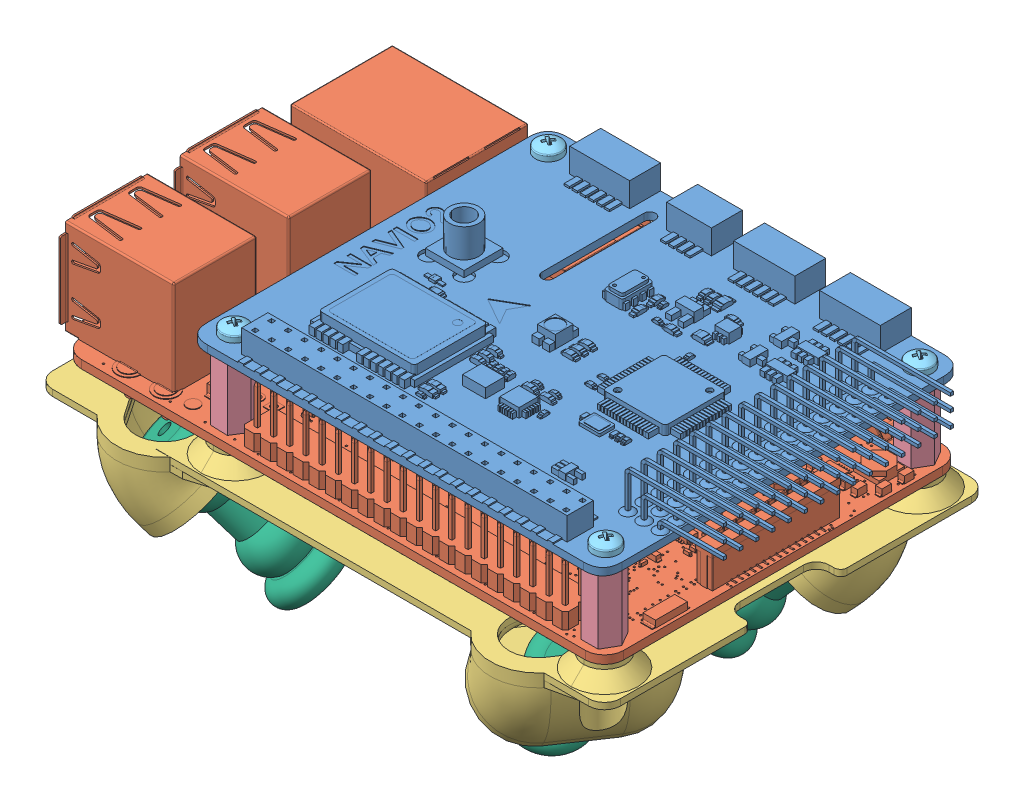
SolidWorks assembly FlightControllerAssembly, configuration Default. Lengths in mm.
Overall size (95.83 50.79 65.38).
19 component instances, 6 part files, 45 mates.
Components (placement in the parent):
- Navio2-1: Navio2 [Predeterminado] at origin size (73.82 8.2 56.43)
- raspberryPi3B-1: raspberryPi3B [Detailed] at (-9.9807 -13.4 -0.0405) x (-1 0 0) z (0 1 0) size (87.05 58.5 19.05)
- VibroNavio2top_rev_A-1: VibroNavio2top_rev_A [Default] at (-9.9807 -17.4 -0.0405) size (89 17.02 65.38)
- Spacer-1: Spacer [Default] at (29.0193 -12.1 24.4595) size (5.4 10.95 4.68)
- Spacer-2: Spacer [Default] at (-28.9807 -12.1 24.4595) x (0.999395 0 0.034774) z (-0.034774 0 0.999395) size (5.4 10.95 4.68)
- Spacer-3: Spacer [Default] at (-28.9807 -12.1 -24.5405) size (5.4 10.95 4.68)
- Spacer-4: Spacer [Default] at (29.0193 -12.1 -24.5405) size (5.4 10.95 4.68)
- pan cross head_am-1: pan cross head_am [B18.6.7M - M2 x 0.4 x 6 Type I Cross Recessed PHMS --6N] at (-28.9807 -17 24.4595) x (0 1 0) z (0 0 1) size (7.58 4 4)
- pan cross head_am-2: pan cross head_am [B18.6.7M - M2 x 0.4 x 6 Type I Cross Recessed PHMS --6N] at (-28.9807 -17 -24.5405) x (0 1 0) z (0 0 1) size (7.58 4 4)
- pan cross head_am-3: pan cross head_am [B18.6.7M - M2 x 0.4 x 6 Type I Cross Recessed PHMS --6N] at (-28.9807 1.6 -24.7405) x (0 -1 0) z (-0.546944 0 0.837169) size (7.58 4 4)
- pan cross head_am-4: pan cross head_am [B18.6.7M - M2 x 0.4 x 6 Type I Cross Recessed PHMS --6N] at (29.0193 -17 -24.5405) x (0 1 0) z (0 0 1) size (7.58 4 4)
- pan cross head_am-5: pan cross head_am [B18.6.7M - M2 x 0.4 x 6 Type I Cross Recessed PHMS --6N] at (29.2193 1.6 -24.7405) x (0 -1 0) z (-0.546944 0 0.837169) size (7.58 4 4)
- pan cross head_am-6: pan cross head_am [B18.6.7M - M2 x 0.4 x 6 Type I Cross Recessed PHMS --6N] at (29.0193 -17 24.4595) x (0 1 0) z (0 0 1) size (7.58 4 4)
- pan cross head_am-7: pan cross head_am [B18.6.7M - M2 x 0.4 x 6 Type I Cross Recessed PHMS --6N] at (29.2193 1.6 24.4595) x (0 -1 0) z (-0.546944 0 0.837169) size (7.58 4 4)
- pan cross head_am-8: pan cross head_am [B18.6.7M - M2 x 0.4 x 6 Type I Cross Recessed PHMS --6N] at (-28.9807 1.6 24.4595) x (0 -1 0) z (-0.546944 0 0.837169) size (7.58 4 4)
- DampeningBall-1: DampeningBall [Default] at (-27.8836 -38.7643 -12.0305) x (0.809631 0.541117 -0.227355) z (-0.054659 0.455184 0.888718) size (12 25 12)
- DampeningBall-2: DampeningBall [Default] at (-27.8836 -38.7643 11.9496) x (0.585019 0.027134 0.810565) z (-0.562354 -0.706586 0.429528) size (12 25 12)
- DampeningBall-3: DampeningBall [Default] at (7.693 -38.5525 11.8752) x (0.798628 -0.586314 -0.135756) z (-0.135756 -0.395268 0.908479) size (12 25 12)
- DampeningBall-4: DampeningBall [Default] at (7.693 -38.5525 -11.9561) x (0.662805 -0.699271 -0.267787) z (0.465753 0.104978 0.878666) size (12 25 12)
Mates (geometry in assembly coordinates):
- Coincident9: coincident aligned: plane of Navio2-1 through (0 0 0) normal (0 0 1)
- Coincident10: coincident aligned: plane of Navio2-1 through (0 0 0) normal (0 1 0)
- Coincident11: coincident aligned: plane of Navio2-1 through (0 0 0) normal (1 0 0)
- Parallel1: parallel aligned: plane of raspberryPi3B-1 through (-9.9807 -13.4 -0.0405) normal (0 1 0)
- Concentric5: concentric aligned: cylinder of Navio2-1 through (-28.9807 -1.166 24.4595) axis (0 1 0) radius 1.3; cylinder of raspberryPi3B-1 through (-28.9807 -13.4 24.4595) axis (0 1 0) radius 1.375
- Parallel3: parallel aligned: plane of Navio2-1 through (-32.5 -1.15 -28.2) normal (0 0 -1); plane of raspberryPi3B-1 through (32.5193 -12.1 -28.0405) normal (0 0 -1)
- Concentric7: concentric anti-aligned: cylinder of raspberryPi3B-1 through (29.0193 -13.4 24.4595) axis (0 1 0) radius 1.375; cylinder of VibroNavio2top_rev_A-1 through (29.0193 -16.4 24.4595) axis (0 -1 0) radius 1.5
- Concentric8: concentric anti-aligned: cylinder of raspberryPi3B-1 through (-28.9807 -13.4 -24.5405) axis (0 1 0) radius 1.375; cylinder of VibroNavio2top_rev_A-1 through (-28.9807 -16.4 -24.5405) axis (0 -1 0) radius 1.5
- Coincident15: coincident anti-aligned: plane of raspberryPi3B-1 through (-9.9807 -13.4 -0.0405) normal (0 -1 0); plane of VibroNavio2top_rev_A-1 through (29.0193 -13.4 -24.5405) normal (0 1 0)
- Concentric9: concentric aligned: cylinder of raspberryPi3B-1 through (-28.9807 -13.4 24.4595) axis (0 1 0) radius 1.375; cylinder of Spacer-2 through (-28.9807 -1.15 24.4595) axis (0 1 0) radius 1.125
- Coincident16: coincident anti-aligned: plane of raspberryPi3B-1 through (-9.9807 -12.1 -0.0405) normal (0 1 0); plane of Spacer-2 through (-28.9807 -12.1 24.4595) normal (0 -1 0)
- Coincident17: coincident anti-aligned: plane of Navio2-1 through (0 -1.15 0) normal (0 -1 0); plane of Spacer-2 through (-28.9807 -1.15 24.4595) normal (0 1 0)
- Concentric10: concentric aligned: cylinder of raspberryPi3B-1 through (29.0193 -13.4 24.4595) axis (0 1 0) radius 1.375; cylinder of Spacer-1 through (29.0193 -1.15 24.4595) axis (0 1 0) radius 1.125
- Coincident18: coincident anti-aligned: plane of Navio2-1 through (0 -1.15 0) normal (0 -1 0); plane of Spacer-1 through (29.0193 -1.15 24.4595) normal (0 1 0)
- Coincident19: coincident anti-aligned: plane of raspberryPi3B-1 through (-9.9807 -12.1 -0.0405) normal (0 1 0); plane of Spacer-1 through (29.0193 -12.1 24.4595) normal (0 -1 0)
- Concentric11: concentric aligned: cylinder of raspberryPi3B-1 through (-28.9807 -13.4 -24.5405) axis (0 1 0) radius 1.375; cylinder of Spacer-3 through (-28.9807 -1.15 -24.5405) axis (0 1 0) radius 1.125
- Coincident20: coincident anti-aligned: plane of Navio2-1 through (0 -1.15 0) normal (0 -1 0); plane of Spacer-3 through (-28.9807 -1.15 -24.5405) normal (0 1 0)
- Coincident21: coincident anti-aligned: plane of raspberryPi3B-1 through (-9.9807 -12.1 -0.0405) normal (0 1 0); plane of Spacer-3 through (-28.9807 -12.1 -24.5405) normal (0 -1 0)
- Concentric12: concentric aligned: cylinder of raspberryPi3B-1 through (29.0193 -13.4 -24.5405) axis (0 1 0) radius 1.375; cylinder of Spacer-4 through (29.0193 -1.15 -24.5405) axis (0 1 0) radius 1.125
- Coincident22: coincident anti-aligned: plane of Navio2-1 through (0 -1.15 0) normal (0 -1 0); plane of Spacer-4 through (29.0193 -1.15 -24.5405) normal (0 1 0)
- Coincident23: coincident anti-aligned: plane of raspberryPi3B-1 through (-9.9807 -12.1 -0.0405) normal (0 1 0); plane of Spacer-4 through (29.0193 -12.1 -24.5405) normal (0 -1 0)
- Concentric17: concentric aligned: cylinder of Navio2-1 through (-28.9807 -1.166 24.4595) axis (0 1 0) radius 1.3; cylinder of pan cross head_am-8 through (-28.9807 27 24.4595) axis (0 1 0) radius 1
- Coincident28: coincident anti-aligned: plane of Navio2-1 through (0 0 0) normal (0 1 0); plane of pan cross head_am-8 through (-28.1435 0 25.0065) normal (0 -1 0)
- Concentric18: concentric anti-aligned: cylinder of Spacer-2 through (-28.9807 -1.15 24.4595) axis (0 1 0) radius 1.125; cylinder of pan cross head_am-1 through (-28.9807 -42.4 24.4595) axis (0 -1 0) radius 1
- Coincident29: coincident anti-aligned: plane of VibroNavio2top_rev_A-1 through (-28.9807 -15.4 24.4595) normal (0 -1 0); plane of pan cross head_am-1 through (-29.9807 -15.4 24.4595) normal (0 1 0)
- Concentric19: concentric aligned: cylinder of Navio2-1 through (29.2193 -1.166 24.4595) axis (0 1 0) radius 1.3; cylinder of pan cross head_am-7 through (29.2193 27 24.4595) axis (0 1 0) radius 1
- Coincident30: coincident anti-aligned: plane of Navio2-1 through (0 0 0) normal (0 1 0); plane of pan cross head_am-7 through (30.0565 0 25.0065) normal (0 -1 0)
- Concentric20: concentric anti-aligned: cylinder of Spacer-1 through (29.0193 -1.15 24.4595) axis (0 1 0) radius 1.125; cylinder of pan cross head_am-6 through (29.0193 -42.4 24.4595) axis (0 -1 0) radius 1
- Coincident31: coincident anti-aligned: plane of VibroNavio2top_rev_A-1 through (29.0193 -15.4 24.4595) normal (0 -1 0); plane of pan cross head_am-6 through (28.0193 -15.4 24.4595) normal (0 1 0)
- Concentric21: concentric aligned: cylinder of Navio2-1 through (29.2193 -1.166 -24.7405) axis (0 1 0) radius 1.3; cylinder of pan cross head_am-5 through (29.2193 27 -24.7405) axis (0 1 0) radius 1
- Coincident32: coincident anti-aligned: plane of Navio2-1 through (0 0 0) normal (0 1 0); plane of pan cross head_am-5 through (30.0565 0 -24.1935) normal (0 -1 0)
- Concentric22: concentric anti-aligned: cylinder of Spacer-4 through (29.0193 -1.15 -24.5405) axis (0 1 0) radius 1.125; cylinder of pan cross head_am-4 through (29.0193 -42.4 -24.5405) axis (0 -1 0) radius 1
- Coincident33: coincident anti-aligned: plane of VibroNavio2top_rev_A-1 through (29.0193 -15.4 -24.5405) normal (0 -1 0); plane of pan cross head_am-4 through (28.0193 -15.4 -24.5405) normal (0 1 0)
- Concentric23: concentric aligned: cylinder of Navio2-1 through (-28.9807 -1.166 -24.7405) axis (0 1 0) radius 1.3; cylinder of pan cross head_am-3 through (-28.9807 27 -24.7405) axis (0 1 0) radius 1
- Coincident34: coincident anti-aligned: plane of Navio2-1 through (0 0 0) normal (0 1 0); plane of pan cross head_am-3 through (-28.1435 0 -24.1935) normal (0 -1 0)
- Concentric24: concentric anti-aligned: cylinder of Spacer-3 through (-28.9807 -1.15 -24.5405) axis (0 1 0) radius 1.125; cylinder of pan cross head_am-2 through (-28.9807 -42.4 -24.5405) axis (0 -1 0) radius 1
- Coincident35: coincident anti-aligned: plane of VibroNavio2top_rev_A-1 through (-28.9807 -15.4 -24.5405) normal (0 -1 0); plane of pan cross head_am-2 through (-29.9807 -15.4 -24.5405) normal (0 1 0)
- Concentric25: concentric anti-aligned: cylinder of VibroNavio2top_rev_A-1 through (-38.9869 -25.3293 19.5136) axis (-0.584389 0.707107 0.398107) radius 5; cylinder of DampeningBall-2 through (-27.8836 -38.7643 11.9496) axis (0.584389 -0.707107 -0.398107) radius 1
- Coincident36: coincident aligned: circle of VibroNavio2top_rev_A-1; plane of DampeningBall-2 through (-40.1557 -23.9151 20.3099) normal (0.584389 -0.707107 -0.398107)
- Concentric26: concentric anti-aligned: cylinder of VibroNavio2top_rev_A-1 through (18.8329 -25.1175 19.3853) axis (0.586314 0.707107 0.395268) radius 5; cylinder of DampeningBall-3 through (7.693 -38.5525 11.8752) axis (-0.586314 -0.707107 -0.395268) radius 1
- Coincident37: coincident aligned: circle of VibroNavio2top_rev_A-1; plane of DampeningBall-3 through (20.0056 -23.7033 20.1758) normal (-0.586314 -0.707107 -0.395268)
- Concentric27: concentric anti-aligned: cylinder of VibroNavio2top_rev_A-1 through (18.8329 -25.1175 -19.4662) axis (0.586314 0.707107 -0.395268) radius 5; cylinder of DampeningBall-4 through (7.693 -38.5525 -11.9561) axis (-0.586314 -0.707107 0.395268) radius 1
- Coincident38: coincident anti-aligned: circle of VibroNavio2top_rev_A-1; plane of DampeningBall-4 through (20.0056 -23.7033 -20.2567) normal (-0.586314 -0.707107 0.395268)
- Concentric28: concentric anti-aligned: cylinder of VibroNavio2top_rev_A-1 through (-38.9869 -25.3293 -19.5946) axis (-0.584389 0.707107 -0.398107) radius 5; cylinder of DampeningBall-1 through (-27.8836 -38.7643 -12.0305) axis (0.584389 -0.707107 0.398107) radius 1
- Coincident39: coincident anti-aligned: circle of VibroNavio2top_rev_A-1; plane of DampeningBall-1 through (-40.1557 -23.9151 -20.3908) normal (0.584389 -0.707107 0.398107)
